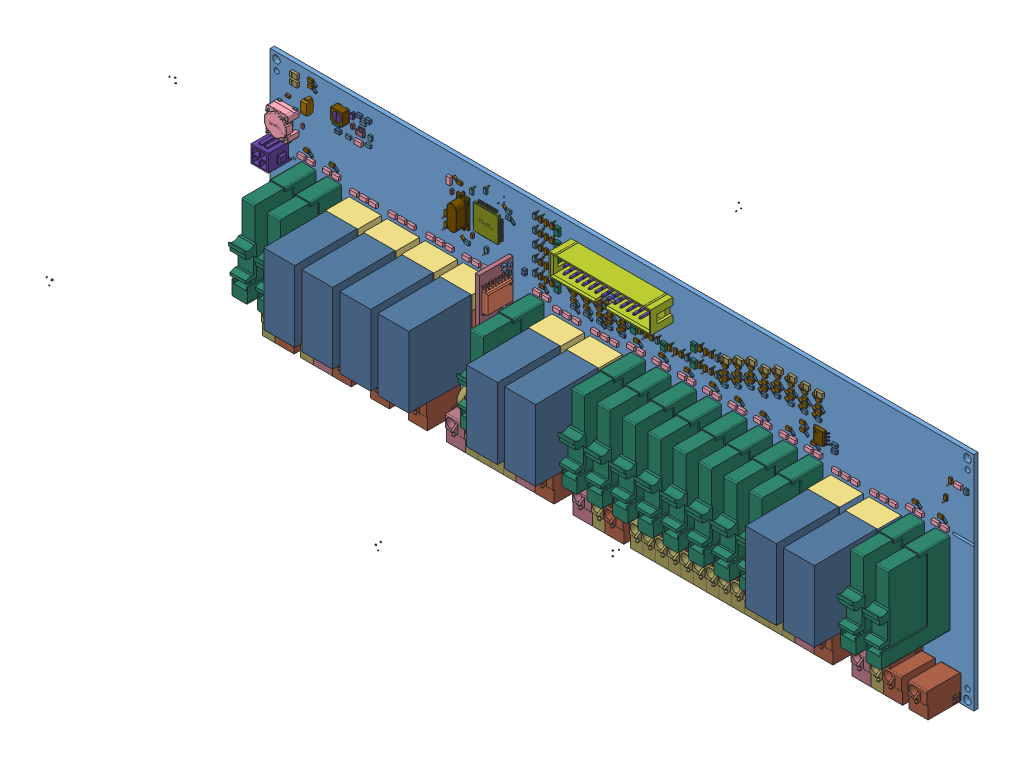
SolidWorks assembly _SC941C, configuration Default. Lengths in mm. (continued)
Components (placement in the parent): (continued)
- T27-1: T27 [Default] at origin size (320.25 73.48 23.48)
  - SW3dPS-transistor_SOT233_4-1: SW3dPS-transistor_SOT233_4 [Default] at (316.7762 70.6118 -21.9) x (1 0 0) z (0 -1 0) size (2.9 1.1 1.6)
  - SW3dPS-transistor_SOT233_5-1: SW3dPS-transistor_SOT233_5 [Default] at (0.3168 0.0706 -0.0219) x (1 0 0) z (0 -1 0) size (2.18 2.18 2.18)
  - SW3dPS-transistor_SOT233_6-1: SW3dPS-transistor_SOT233_6 [Default] at (0.0003 0.0001 0) x (1 0 0) z (0 -1 0) size (2.18 2.18 2.18)
  - SW3dPS-transistor_SOT233_7-1: SW3dPS-transistor_SOT233_7 [Default] x (1 0 0) z (0 -1 0) size (2.18 2.18 2.18)
- T24-1: T24 [Default] at origin size (297.39 73.44 23.48)
  - SW3dPS-transistor_SOT233_4-1: SW3dPS-transistor_SOT233_4 [Default] at (293.9162 70.5668 -21.9) x (1 0 0) z (0 -1 0) size (2.9 1.1 1.6)
  - SW3dPS-transistor_SOT233_5-1: SW3dPS-transistor_SOT233_5 [Default] at (0.2939 0.0706 -0.0219) x (1 0 0) z (0 -1 0) size (2.18 2.18 2.18)
  - SW3dPS-transistor_SOT233_6-1: SW3dPS-transistor_SOT233_6 [Default] at (0.0003 0.0001 0) x (1 0 0) z (0 -1 0) size (2.18 2.18 2.18)
  - SW3dPS-transistor_SOT233_7-1: SW3dPS-transistor_SOT233_7 [Default] x (1 0 0) z (0 -1 0) size (2.18 2.18 2.18)
- T25-1: T25 [Default] at origin size (305.01 73.44 23.48)
  - SW3dPS-transistor_SOT233_4-1: SW3dPS-transistor_SOT233_4 [Default] at (301.5362 70.5668 -21.9) x (1 0 0) z (0 -1 0) size (2.9 1.1 1.6)
  - SW3dPS-transistor_SOT233_5-1: SW3dPS-transistor_SOT233_5 [Default] at (0.3015 0.0706 -0.0219) x (1 0 0) z (0 -1 0) size (2.18 2.18 2.18)
  - SW3dPS-transistor_SOT233_6-1: SW3dPS-transistor_SOT233_6 [Default] at (0.0003 0.0001 0) x (1 0 0) z (0 -1 0) size (2.18 2.18 2.18)
  - SW3dPS-transistor_SOT233_7-1: SW3dPS-transistor_SOT233_7 [Default] x (1 0 0) z (0 -1 0) size (2.18 2.18 2.18)
- T14-1: T14 [Default] at origin size (200.87 73.48 23.48)
  - SW3dPS-transistor_SOT233_4-1: SW3dPS-transistor_SOT233_4 [Default] at (197.3962 70.6118 -21.9) x (1 0 0) z (0 -1 0) size (2.9 1.1 1.6)
  - SW3dPS-transistor_SOT233_5-1: SW3dPS-transistor_SOT233_5 [Default] at (0.1974 0.0706 -0.0219) x (1 0 0) z (0 -1 0) size (2.18 2.18 2.18)
  - SW3dPS-transistor_SOT233_6-1: SW3dPS-transistor_SOT233_6 [Default] at (0.0002 0.0001 0) x (1 0 0) z (0 -1 0) size (2.18 2.18 2.18)
  - SW3dPS-transistor_SOT233_7-1: SW3dPS-transistor_SOT233_7 [Default] x (1 0 0) z (0 -1 0) size (2.18 2.18 2.18)
- T15-1: T15 [Default] at origin size (208.49 73.48 23.48)
  - SW3dPS-transistor_SOT233_4-1: SW3dPS-transistor_SOT233_4 [Default] at (205.0162 70.6118 -21.9) x (1 0 0) z (0 -1 0) size (2.9 1.1 1.6)
  - SW3dPS-transistor_SOT233_5-1: SW3dPS-transistor_SOT233_5 [Default] at (0.205 0.0706 -0.0219) x (1 0 0) z (0 -1 0) size (2.18 2.18 2.18)
  - SW3dPS-transistor_SOT233_6-1: SW3dPS-transistor_SOT233_6 [Default] at (0.0002 0.0001 0) x (1 0 0) z (0 -1 0) size (2.18 2.18 2.18)
  - SW3dPS-transistor_SOT233_7-1: SW3dPS-transistor_SOT233_7 [Default] x (1 0 0) z (0 -1 0) size (2.18 2.18 2.18)
- T12-1: T12 [Default] at origin size (185.63 73.48 23.48)
  - SW3dPS-transistor_SOT233_4-1: SW3dPS-transistor_SOT233_4 [Default] at (182.1562 70.6118 -21.9) x (1 0 0) z (0 -1 0) size (2.9 1.1 1.6)
  - SW3dPS-transistor_SOT233_5-1: SW3dPS-transistor_SOT233_5 [Default] at (0.1822 0.0706 -0.0219) x (1 0 0) z (0 -1 0) size (2.18 2.18 2.18)
  - SW3dPS-transistor_SOT233_6-1: SW3dPS-transistor_SOT233_6 [Default] at (0.0002 0.0001 0) x (1 0 0) z (0 -1 0) size (2.18 2.18 2.18)
  - SW3dPS-transistor_SOT233_7-1: SW3dPS-transistor_SOT233_7 [Default] x (1 0 0) z (0 -1 0) size (2.18 2.18 2.18)
- T13-1: T13 [Default] at origin size (193.25 73.48 23.48)
  - SW3dPS-transistor_SOT233_4-1: SW3dPS-transistor_SOT233_4 [Default] at (189.7762 70.6118 -21.9) x (1 0 0) z (0 -1 0) size (2.9 1.1 1.6)
  - SW3dPS-transistor_SOT233_5-1: SW3dPS-transistor_SOT233_5 [Default] at (0.1898 0.0706 -0.0219) x (1 0 0) z (0 -1 0) size (2.18 2.18 2.18)
  - SW3dPS-transistor_SOT233_6-1: SW3dPS-transistor_SOT233_6 [Default] at (0.0002 0.0001 0) x (1 0 0) z (0 -1 0) size (2.18 2.18 2.18)
  - SW3dPS-transistor_SOT233_7-1: SW3dPS-transistor_SOT233_7 [Default] x (1 0 0) z (0 -1 0) size (2.18 2.18 2.18)
- T9-1: T9 [Default] at origin size (149.28 73.48 23.48)
  - SW3dPS-transistor_SOT233_4-1: SW3dPS-transistor_SOT233_4 [Default] at (145.8024 70.6118 -21.9) x (1 0 0) z (0 -1 0) size (2.9 1.1 1.6)
  - SW3dPS-transistor_SOT233_5-1: SW3dPS-transistor_SOT233_5 [Default] at (0.1458 0.0706 -0.0219) x (1 0 0) z (0 -1 0) size (2.18 2.18 2.18)
  - SW3dPS-transistor_SOT233_6-1: SW3dPS-transistor_SOT233_6 [Default] at (0.0001 0.0001 0) x (1 0 0) z (0 -1 0) size (2.18 2.18 2.18)
  - SW3dPS-transistor_SOT233_7-1: SW3dPS-transistor_SOT233_7 [Default] x (1 0 0) z (0 -1 0) size (2.18 2.18 2.18)
- T10-1: T10 [Default] at origin size (156.9 73.48 23.48)
  - SW3dPS-transistor_SOT233_4-1: SW3dPS-transistor_SOT233_4 [Default] at (153.4224 70.6118 -21.9) x (1 0 0) z (0 -1 0) size (2.9 1.1 1.6)
  - SW3dPS-transistor_SOT233_5-1: SW3dPS-transistor_SOT233_5 [Default] at (0.1534 0.0706 -0.0219) x (1 0 0) z (0 -1 0) size (2.18 2.18 2.18)
  - SW3dPS-transistor_SOT233_6-1: SW3dPS-transistor_SOT233_6 [Default] at (0.0002 0.0001 0) x (1 0 0) z (0 -1 0) size (2.18 2.18 2.18)
  - SW3dPS-transistor_SOT233_7-1: SW3dPS-transistor_SOT233_7 [Default] x (1 0 0) z (0 -1 0) size (2.18 2.18 2.18)
- T7_1-1: T7_1 [Default] at origin size (134.83 73.44 23.48)
  - SW3dPS-transistor_SOT233_4-1: SW3dPS-transistor_SOT233_4 [Default] at (131.3562 70.5668 -21.9) x (1 0 0) z (0 -1 0) size (2.9 1.1 1.6)
  - SW3dPS-transistor_SOT233_5-1: SW3dPS-transistor_SOT233_5 [Default] at (0.1314 0.0706 -0.0219) x (1 0 0) z (0 -1 0) size (2.18 2.18 2.18)
  - SW3dPS-transistor_SOT233_6-1: SW3dPS-transistor_SOT233_6 [Default] at (0.0001 0.0001 0) x (1 0 0) z (0 -1 0) size (2.18 2.18 2.18)
  - SW3dPS-transistor_SOT233_7-1: SW3dPS-transistor_SOT233_7 [Default] x (1 0 0) z (0 -1 0) size (2.18 2.18 2.18)
- T8-1: T8 [Default] at origin size (142.45 73.44 23.48)
  - SW3dPS-transistor_SOT233_4-1: SW3dPS-transistor_SOT233_4 [Default] at (138.9762 70.5668 -21.9) x (1 0 0) z (0 -1 0) size (2.9 1.1 1.6)
  - SW3dPS-transistor_SOT233_5-1: SW3dPS-transistor_SOT233_5 [Default] at (0.139 0.0706 -0.0219) x (1 0 0) z (0 -1 0) size (2.18 2.18 2.18)
  - SW3dPS-transistor_SOT233_6-1: SW3dPS-transistor_SOT233_6 [Default] at (0.0001 0.0001 0) x (1 0 0) z (0 -1 0) size (2.18 2.18 2.18)
  - SW3dPS-transistor_SOT233_7-1: SW3dPS-transistor_SOT233_7 [Default] x (1 0 0) z (0 -1 0) size (2.18 2.18 2.18)
- T5_1-1: T5_1 [Default] at origin size (119.59 73.44 23.48)
  - SW3dPS-transistor_SOT233_4-1: SW3dPS-transistor_SOT233_4 [Default] at (116.1162 70.5668 -21.9) x (1 0 0) z (0 -1 0) size (2.9 1.1 1.6)
  - SW3dPS-transistor_SOT233_5-1: SW3dPS-transistor_SOT233_5 [Default] at (0.1161 0.0706 -0.0219) x (1 0 0) z (0 -1 0) size (2.18 2.18 2.18)
  - SW3dPS-transistor_SOT233_6-1: SW3dPS-transistor_SOT233_6 [Default] at (0.0001 0.0001 0) x (1 0 0) z (0 -1 0) size (2.18 2.18 2.18)
  - SW3dPS-transistor_SOT233_7-1: SW3dPS-transistor_SOT233_7 [Default] x (1 0 0) z (0 -1 0) size (2.18 2.18 2.18)
- T6_1-1: T6_1 [Default] at origin size (127.21 73.44 23.48)
  - SW3dPS-transistor_SOT233_4-1: SW3dPS-transistor_SOT233_4 [Default] at (123.7362 70.5668 -21.9) x (1 0 0) z (0 -1 0) size (2.9 1.1 1.6)
  - SW3dPS-transistor_SOT233_5-1: SW3dPS-transistor_SOT233_5 [Default] at (0.1237 0.0706 -0.0219) x (1 0 0) z (0 -1 0) size (2.18 2.18 2.18)
  - SW3dPS-transistor_SOT233_6-1: SW3dPS-transistor_SOT233_6 [Default] at (0.0001 0.0001 0) x (1 0 0) z (0 -1 0) size (2.18 2.18 2.18)
  - SW3dPS-transistor_SOT233_7-1: SW3dPS-transistor_SOT233_7 [Default] x (1 0 0) z (0 -1 0) size (2.18 2.18 2.18)
- T3_1-1: T3_1 [Default] at origin size (104.35 73.44 23.48)
  - SW3dPS-transistor_SOT233_4-1: SW3dPS-transistor_SOT233_4 [Default] at (100.8762 70.5668 -21.9) x (1 0 0) z (0 -1 0) size (2.9 1.1 1.6)
  - SW3dPS-transistor_SOT233_5-1: SW3dPS-transistor_SOT233_5 [Default] at (0.1009 0.0706 -0.0219) x (1 0 0) z (0 -1 0) size (2.18 2.18 2.18)
  - SW3dPS-transistor_SOT233_6-1: SW3dPS-transistor_SOT233_6 [Default] at (0.0001 0.0001 0) x (1 0 0) z (0 -1 0) size (2.18 2.18 2.18)
  - SW3dPS-transistor_SOT233_7-1: SW3dPS-transistor_SOT233_7 [Default] x (1 0 0) z (0 -1 0) size (2.18 2.18 2.18)
- SUP_K19-1: SUP_K19 [Default] at origin size (13 30.3 9.5)
  - 1151724792-1: 1151724792 [Default] at (240.665 37.325 0) size (13 14.8 9.5)
    - Extruded_5-1: Extruded_5 [Default] at origin size (13 14.8 9.5)
  - 1151725064-1: 1151725064 [Default] at (240.665 24.925 5) size (13 10 4.5)
    - Extruded_6-1: Extruded_6 [Default] at origin size (13 10 4.5)
  - 1151724928-1: 1151724928 [Default] at (240.665 17.175 0) size (13 5.5 9.5)
    - Extruded_7-1: Extruded_7 [Default] at origin size (13 5.5 9.5)
- SUP_K18-1: SUP_K18 [Default] at origin size (13 30.3 9.5)
  - 1151724792-1: 1151724792 [Default] at (225.425 37.325 0) size (13 14.8 9.5)
    - Extruded_5-1: Extruded_5 [Default] at origin size (13 14.8 9.5)
  - 1151725064-1: 1151725064 [Default] at (225.425 24.925 5) size (13 10 4.5)
    - Extruded_6-1: Extruded_6 [Default] at origin size (13 10 4.5)
  - 1151724928-1: 1151724928 [Default] at (225.425 17.175 0) size (13 5.5 9.5)
    - Extruded_7-1: Extruded_7 [Default] at origin size (13 5.5 9.5)
- SUP_K6-1: SUP_K6 [Default] at origin size (13 30.3 9.5)
  - 1151724792-1: 1151724792 [Default] at (78.105 21.825 0) size (13 14.8 9.5)
    - Extruded_5-1: Extruded_5 [Default] at origin size (13 14.8 9.5)
  - 1151725064-1: 1151725064 [Default] at (78.105 34.225 5) size (13 10 4.5)
    - Extruded_6-1: Extruded_6 [Default] at origin size (13 10 4.5)
  - 1151724928-1: 1151724928 [Default] at (78.105 41.975 0) size (13 5.5 9.5)
    - Extruded_7-1: Extruded_7 [Default] at origin size (13 5.5 9.5)
- SUP_K5-1: SUP_K5 [Default] at origin size (13 30.3 9.5)
  - 1151724792-1: 1151724792 [Default] at (62.865 21.825 0) size (13 14.8 9.5)
    - Extruded_5-1: Extruded_5 [Default] at origin size (13 14.8 9.5)
  - 1151725064-1: 1151725064 [Default] at (62.865 34.225 5) size (13 10 4.5)
    - Extruded_6-1: Extruded_6 [Default] at origin size (13 10 4.5)
  - 1151724928-1: 1151724928 [Default] at (62.865 41.975 0) size (13 5.5 9.5)
    - Extruded_7-1: Extruded_7 [Default] at origin size (13 5.5 9.5)
- SUP_K4-1: SUP_K4 [Default] at origin size (13 30.3 9.5)
  - 1151724792-1: 1151724792 [Default] at (47.625 21.825 0) size (13 14.8 9.5)
    - Extruded_5-1: Extruded_5 [Default] at origin size (13 14.8 9.5)
  - 1151725064-1: 1151725064 [Default] at (47.625 34.225 5) size (13 10 4.5)
    - Extruded_6-1: Extruded_6 [Default] at origin size (13 10 4.5)
  - 1151724928-1: 1151724928 [Default] at (47.625 41.975 0) size (13 5.5 9.5)
    - Extruded_7-1: Extruded_7 [Default] at origin size (13 5.5 9.5)
- SUP_K3-1: SUP_K3 [Default] at origin size (13 30.3 9.5)
  - 1151724792-1: 1151724792 [Default] at (32.385 21.825 0) size (13 14.8 9.5)
    - Extruded_5-1: Extruded_5 [Default] at origin size (13 14.8 9.5)
  - 1151725064-1: 1151725064 [Default] at (32.385 34.225 5) size (13 10 4.5)
    - Extruded_6-1: Extruded_6 [Default] at origin size (13 10 4.5)
  - 1151724928-1: 1151724928 [Default] at (32.385 41.975 0) size (13 5.5 9.5)
    - Extruded_7-1: Extruded_7 [Default] at origin size (13 5.5 9.5)
- R86-1: R86 [Default] at origin size (3.3 1.97 0.78)
  - SW3dPS-0805_SMD_Resistor-1: SW3dPS-0805_SMD_Resistor [Default] at (192.7859 64.1349 0) x (-1 0 0) z (0 1 0) size (2 0.78 1.25)
  - 905261096-1: 905261096 [Default] at (194.5719 63.4603 0) size (1.03 1.35 0.76)
    - Extruded_2-1: Extruded_2 [Default] at origin size (1.03 1.35 0.76)
  - 905275240-1: 905275240 [Default] at (194.3338 63.5397 0) size (1.51 1.51 0.76)
    - Extruded_3-1: Extruded_3 [Default] at origin size (1.51 1.51 0.76)
  - 905265720-1: 905265720 [Default] at (194.4529 63.5 0) size (1.11 1.43 0.76)
    - Extruded_4-1: Extruded_4 [Default] at origin size (1.11 1.43 0.76)
- R82-1: R82 [Default] at origin size (3.3 1.97 0.78)
  - SW3dPS-0805_SMD_Resistor-1: SW3dPS-0805_SMD_Resistor [Default] at (197.9929 66.4209 0) x (-1 0 0) z (0 1 0) size (2 0.78 1.25)
  - 905261096-1: 905261096 [Default] at (199.7789 65.7463 0) size (1.03 1.35 0.76)
    - Extruded_2-1: Extruded_2 [Default] at origin size (1.03 1.35 0.76)
  - 905275240-1: 905275240 [Default] at (199.5408 65.8257 0) size (1.51 1.51 0.76)
    - Extruded_3-1: Extruded_3 [Default] at origin size (1.51 1.51 0.76)
  - 905265720-1: 905265720 [Default] at (199.6599 65.786 0) size (1.11 1.43 0.76)
    - Extruded_4-1: Extruded_4 [Default] at origin size (1.11 1.43 0.76)
- R90-1: R90 [Default] at origin size (1.97 3.3 0.78)
  - SW3dPS-0805_SMD_Resistor-1: SW3dPS-0805_SMD_Resistor [Default] at (265.4299 60.3251 0) x (0 1 0) z (1 0 0) size (2 0.78 1.25)
  - 905261640-1: 905261640 [Default] at (264.7553 58.5391 0) size (1.35 1.03 0.76)
    - Extruded_8-1: Extruded_8 [Default] at origin size (1.35 1.03 0.76)
  - 905260416-1: 905260416 [Default] at (264.8347 58.7772 0) size (1.51 1.51 0.76)
    - Extruded_9-1: Extruded_9 [Default] at origin size (1.51 1.51 0.76)
  - 905266128-1: 905266128 [Default] at (264.795 58.6581 0) size (1.43 1.11 0.76)
    - Extruded_10-1: Extruded_10 [Default] at origin size (1.43 1.11 0.76)
- R42-1: R42 [Default] at origin size (3.3 1.97 0.78)
  - SW3dPS-0805_SMD_Resistor-1: SW3dPS-0805_SMD_Resistor [Default] at (70.6121 72.1361 0) x (1 0 0) z (0 -1 0) size (2 0.78 1.25)
  - 905266264-1: 905266264 [Default] at (68.8261 72.8107 0) size (1.03 1.35 0.76)
    - Extruded_14-1: Extruded_14 [Default] at origin size (1.03 1.35 0.76)
  - 905263816-1: 905263816 [Default] at (69.0642 72.7313 0) size (1.51 1.51 0.76)
    - Extruded_15-1: Extruded_15 [Default] at origin size (1.51 1.51 0.76)
  - 905266536-1: 905266536 [Default] at (68.9451 72.771 0) size (1.11 1.43 0.76)
    - Extruded_16-1: Extruded_16 [Default] at origin size (1.11 1.43 0.76)
- R43-1: R43 [Default] at origin size (1.97 3.3 0.78)
  - SW3dPS-0805_SMD_Resistor-1: SW3dPS-0805_SMD_Resistor [Default] at (65.1509 54.8641 0) x (0 1 0) z (1 0 0) size (2 0.78 1.25)
  - 905261640-1: 905261640 [Default] at (64.4763 53.0781 0) size (1.35 1.03 0.76)
    - Extruded_8-1: Extruded_8 [Default] at origin size (1.35 1.03 0.76)
  - 905260416-1: 905260416 [Default] at (64.5557 53.3162 0) size (1.51 1.51 0.76)
    - Extruded_9-1: Extruded_9 [Default] at origin size (1.51 1.51 0.76)
  - 905266128-1: 905266128 [Default] at (64.516 53.1971 0) size (1.43 1.11 0.76)
    - Extruded_10-1: Extruded_10 [Default] at origin size (1.43 1.11 0.76)
- R44-1: R44 [Default] at origin size (1.97 3.3 0.78)
  - SW3dPS-0805_SMD_Resistor-1: SW3dPS-0805_SMD_Resistor [Default] at (65.1509 58.9281 0) x (0 1 0) z (1 0 0) size (2 0.78 1.25)
  - 905261640-1: 905261640 [Default] at (64.4763 57.1421 0) size (1.35 1.03 0.76)
    - Extruded_8-1: Extruded_8 [Default] at origin size (1.35 1.03 0.76)
  - 905260416-1: 905260416 [Default] at (64.5557 57.3802 0) size (1.51 1.51 0.76)
    - Extruded_9-1: Extruded_9 [Default] at origin size (1.51 1.51 0.76)
  - 905266128-1: 905266128 [Default] at (64.516 57.2611 0) size (1.43 1.11 0.76)
    - Extruded_10-1: Extruded_10 [Default] at origin size (1.43 1.11 0.76)
- R91-1: R91 [Default] at origin size (1.97 3.3 0.78)
  - SW3dPS-0805_SMD_Resistor-1: SW3dPS-0805_SMD_Resistor [Default] at (267.3349 67.1513 0) x (0 1 0) z (1 0 0) size (2 0.78 1.25)
  - 905261640-1: 905261640 [Default] at (266.6603 65.3653 0) size (1.35 1.03 0.76)
    - Extruded_8-1: Extruded_8 [Default] at origin size (1.35 1.03 0.76)
  - 905260416-1: 905260416 [Default] at (266.7397 65.6034 0) size (1.51 1.51 0.76)
    - Extruded_9-1: Extruded_9 [Default] at origin size (1.51 1.51 0.76)
  - 905266128-1: 905266128 [Default] at (266.7 65.4844 0) size (1.43 1.11 0.76)
    - Extruded_10-1: Extruded_10 [Default] at origin size (1.43 1.11 0.76)
- R87-1: R87 [Default] at origin size (3.3 1.97 0.78)
  - SW3dPS-0805_SMD_Resistor-1: SW3dPS-0805_SMD_Resistor [Default] at (192.7861 61.8491 0) x (1 0 0) z (0 -1 0) size (2 0.78 1.25)
  - 905266264-1: 905266264 [Default] at (191.0001 62.5237 0) size (1.03 1.35 0.76)
    - Extruded_14-1: Extruded_14 [Default] at origin size (1.03 1.35 0.76)
  - 905263816-1: 905263816 [Default] at (191.2382 62.4443 0) size (1.51 1.51 0.76)
    - Extruded_15-1: Extruded_15 [Default] at origin size (1.51 1.51 0.76)
  - 905266536-1: 905266536 [Default] at (191.1191 62.484 0) size (1.11 1.43 0.76)
    - Extruded_16-1: Extruded_16 [Default] at origin size (1.11 1.43 0.76)
- R83-1: R83 [Default] at origin size (3.3 1.97 0.78)
  - SW3dPS-0805_SMD_Resistor-1: SW3dPS-0805_SMD_Resistor [Default] at (197.9931 64.1351 0) x (1 0 0) z (0 -1 0) size (2 0.78 1.25)
  - 905266264-1: 905266264 [Default] at (196.2071 64.8097 0) size (1.03 1.35 0.76)
    - Extruded_14-1: Extruded_14 [Default] at origin size (1.03 1.35 0.76)
  - 905263816-1: 905263816 [Default] at (196.4452 64.7303 0) size (1.51 1.51 0.76)
    - Extruded_15-1: Extruded_15 [Default] at origin size (1.51 1.51 0.76)
  - 905266536-1: 905266536 [Default] at (196.3261 64.77 0) size (1.11 1.43 0.76)
    - Extruded_16-1: Extruded_16 [Default] at origin size (1.11 1.43 0.76)
- R88-1: R88 [Default] at origin size (3.3 1.97 0.78)
  - SW3dPS-0805_SMD_Resistor-1: SW3dPS-0805_SMD_Resistor [Default] at (192.7861 66.4211 0) x (1 0 0) z (0 -1 0) size (2 0.78 1.25)
  - 905266264-1: 905266264 [Default] at (191.0001 67.0957 0) size (1.03 1.35 0.76)
    - Extruded_14-1: Extruded_14 [Default] at origin size (1.03 1.35 0.76)
  - 905263816-1: 905263816 [Default] at (191.2382 67.0163 0) size (1.51 1.51 0.76)
    - Extruded_15-1: Extruded_15 [Default] at origin size (1.51 1.51 0.76)
  - 905266536-1: 905266536 [Default] at (191.1191 67.056 0) size (1.11 1.43 0.76)
    - Extruded_16-1: Extruded_16 [Default] at origin size (1.11 1.43 0.76)
- R84-1: R84 [Default] at origin size (3.3 1.97 0.78)
  - SW3dPS-0805_SMD_Resistor-1: SW3dPS-0805_SMD_Resistor [Default] at (197.9931 68.7071 0) x (1 0 0) z (0 -1 0) size (2 0.78 1.25)
  - 905266264-1: 905266264 [Default] at (196.2071 69.3817 0) size (1.03 1.35 0.76)
    - Extruded_14-1: Extruded_14 [Default] at origin size (1.03 1.35 0.76)
  - 905263816-1: 905263816 [Default] at (196.4452 69.3023 0) size (1.51 1.51 0.76)
    - Extruded_15-1: Extruded_15 [Default] at origin size (1.51 1.51 0.76)
  - 905266536-1: 905266536 [Default] at (196.3261 69.342 0) size (1.11 1.43 0.76)
    - Extruded_16-1: Extruded_16 [Default] at origin size (1.11 1.43 0.76)
- R3_1-1: R3_1 [Default] at origin size (3.3 1.97 0.78)
  - SW3dPS-0805_SMD_Resistor-1: SW3dPS-0805_SMD_Resistor [Default] at (10.8267 75.7079 0) x (-1 0 0) z (0 1 0) size (2 0.78 1.25)
  - 905261096-1: 905261096 [Default] at (12.6127 75.0333 0) size (1.03 1.35 0.76)
    - Extruded_2-1: Extruded_2 [Default] at origin size (1.03 1.35 0.76)
  - 905275240-1: 905275240 [Default] at (12.3746 75.1127 0) size (1.51 1.51 0.76)
    - Extruded_3-1: Extruded_3 [Default] at origin size (1.51 1.51 0.76)
  - 905265720-1: 905265720 [Default] at (12.4936 75.073 0) size (1.11 1.43 0.76)
    - Extruded_4-1: Extruded_4 [Default] at origin size (1.11 1.43 0.76)
- R1_1-1: R1_1 [Default] at origin size (3.3 1.97 0.78)
  - SW3dPS-0805_SMD_Resistor-1: SW3dPS-0805_SMD_Resistor [Default] at (10.8267 77.7716 0) x (-1 0 0) z (0 1 0) size (2 0.78 1.25)
  - 905261096-1: 905261096 [Default] at (12.6127 77.0971 0) size (1.03 1.35 0.76)
    - Extruded_2-1: Extruded_2 [Default] at origin size (1.03 1.35 0.76)
  - 905275240-1: 905275240 [Default] at (12.3746 77.1764 0) size (1.51 1.51 0.76)
    - Extruded_3-1: Extruded_3 [Default] at origin size (1.51 1.51 0.76)
  - 905265720-1: 905265720 [Default] at (12.4936 77.1367 0) size (1.11 1.43 0.76)
    - Extruded_4-1: Extruded_4 [Default] at origin size (1.11 1.43 0.76)
- R79-1: R79 [Default] at origin size (3.3 1.97 0.78)
  - SW3dPS-0805_SMD_Resistor-1: SW3dPS-0805_SMD_Resistor [Default] at (187.3249 64.1349 0) x (-1 0 0) z (0 1 0) size (2 0.78 1.25)
  - 905261096-1: 905261096 [Default] at (189.1109 63.4603 0) size (1.03 1.35 0.76)
    - Extruded_2-1: Extruded_2 [Default] at origin size (1.03 1.35 0.76)
  - 905275240-1: 905275240 [Default] at (188.8728 63.5397 0) size (1.51 1.51 0.76)
    - Extruded_3-1: Extruded_3 [Default] at origin size (1.51 1.51 0.76)
  - 905265720-1: 905265720 [Default] at (188.9919 63.5 0) size (1.11 1.43 0.76)
    - Extruded_4-1: Extruded_4 [Default] at origin size (1.11 1.43 0.76)
- R46-1: R46 [Default] at origin size (1.97 3.3 0.78)
  - SW3dPS-0805_SMD_Resistor-1: SW3dPS-0805_SMD_Resistor [Default] at (157.0989 56.8961 0) x (0 1 0) z (1 0 0) size (2 0.78 1.25)
  - 905261640-1: 905261640 [Default] at (156.4243 55.1101 0) size (1.35 1.03 0.76)
    - Extruded_8-1: Extruded_8 [Default] at origin size (1.35 1.03 0.76)
  - 905260416-1: 905260416 [Default] at (156.5037 55.3482 0) size (1.51 1.51 0.76)
    - Extruded_9-1: Extruded_9 [Default] at origin size (1.51 1.51 0.76)
  - 905266128-1: 905266128 [Default] at (156.464 55.2291 0) size (1.43 1.11 0.76)
    - Extruded_10-1: Extruded_10 [Default] at origin size (1.43 1.11 0.76)
- R29-1: R29 [Default] at origin size (3.3 1.97 0.78)
  - SW3dPS-0805_SMD_Resistor-1: SW3dPS-0805_SMD_Resistor [Default] at (126.6191 56.5151 0) x (1 0 0) z (0 -1 0) size (2 0.78 1.25)
  - 905266264-1: 905266264 [Default] at (124.8331 57.1897 0) size (1.03 1.35 0.76)
    - Extruded_14-1: Extruded_14 [Default] at origin size (1.03 1.35 0.76)
  - 905263816-1: 905263816 [Default] at (125.0712 57.1103 0) size (1.51 1.51 0.76)
    - Extruded_15-1: Extruded_15 [Default] at origin size (1.51 1.51 0.76)
  - 905266536-1: 905266536 [Default] at (124.9521 57.15 0) size (1.11 1.43 0.76)
    - Extruded_16-1: Extruded_16 [Default] at origin size (1.11 1.43 0.76)
- R31-1: R31 [Default] at origin size (1.97 3.3 0.78)
  - SW3dPS-0805_SMD_Resistor-1: SW3dPS-0805_SMD_Resistor [Default] at (105.2829 55.7531 0) x (0 1 0) z (1 0 0) size (2 0.78 1.25)
  - 905261640-1: 905261640 [Default] at (104.6083 53.9671 0) size (1.35 1.03 0.76)
    - Extruded_8-1: Extruded_8 [Default] at origin size (1.35 1.03 0.76)
  - 905260416-1: 905260416 [Default] at (104.6877 54.2052 0) size (1.51 1.51 0.76)
    - Extruded_9-1: Extruded_9 [Default] at origin size (1.51 1.51 0.76)
  - 905266128-1: 905266128 [Default] at (104.648 54.0861 0) size (1.43 1.11 0.76)
    - Extruded_10-1: Extruded_10 [Default] at origin size (1.43 1.11 0.76)
- R24-1: R24 [Default] at origin size (1.97 3.3 0.78)
  - SW3dPS-0805_SMD_Resistor-1: SW3dPS-0805_SMD_Resistor [Default] at (105.2829 75.5651 0) x (0 1 0) z (1 0 0) size (2 0.78 1.25)
  - 905261640-1: 905261640 [Default] at (104.6083 73.7791 0) size (1.35 1.03 0.76)
    - Extruded_8-1: Extruded_8 [Default] at origin size (1.35 1.03 0.76)
  - 905260416-1: 905260416 [Default] at (104.6877 74.0172 0) size (1.51 1.51 0.76)
    - Extruded_9-1: Extruded_9 [Default] at origin size (1.51 1.51 0.76)
  - 905266128-1: 905266128 [Default] at (104.648 73.8981 0) size (1.43 1.11 0.76)
    - Extruded_10-1: Extruded_10 [Default] at origin size (1.43 1.11 0.76)
- R19_1-1: R19_1 [Default] at origin size (1.97 3.3 0.78)
  - SW3dPS-0805_SMD_Resistor-1: SW3dPS-0805_SMD_Resistor [Default] at (105.2829 65.6591 0) x (0 1 0) z (1 0 0) size (2 0.78 1.25)
  - 905261640-1: 905261640 [Default] at (104.6083 63.8731 0) size (1.35 1.03 0.76)
    - Extruded_8-1: Extruded_8 [Default] at origin size (1.35 1.03 0.76)
  - 905260416-1: 905260416 [Default] at (104.6877 64.1112 0) size (1.51 1.51 0.76)
    - Extruded_9-1: Extruded_9 [Default] at origin size (1.51 1.51 0.76)
  - 905266128-1: 905266128 [Default] at (104.648 63.9921 0) size (1.43 1.11 0.76)
    - Extruded_10-1: Extruded_10 [Default] at origin size (1.43 1.11 0.76)
- R13-1: R13 [Default] at origin size (1.97 3.3 0.78)
  - SW3dPS-0805_SMD_Resistor-1: SW3dPS-0805_SMD_Resistor [Default] at (105.2829 70.6121 0) x (0 1 0) z (1 0 0) size (2 0.78 1.25)
  - 905261640-1: 905261640 [Default] at (104.6083 68.8261 0) size (1.35 1.03 0.76)
    - Extruded_8-1: Extruded_8 [Default] at origin size (1.35 1.03 0.76)
  - 905260416-1: 905260416 [Default] at (104.6877 69.0642 0) size (1.51 1.51 0.76)
    - Extruded_9-1: Extruded_9 [Default] at origin size (1.51 1.51 0.76)
  - 905266128-1: 905266128 [Default] at (104.648 68.9451 0) size (1.43 1.11 0.76)
    - Extruded_10-1: Extruded_10 [Default] at origin size (1.43 1.11 0.76)
- R76-1: R76 [Default] at origin size (3.3 1.97 0.78)
  - SW3dPS-0805_SMD_Resistor-1: SW3dPS-0805_SMD_Resistor [Default] at (203.4539 66.4209 0) x (-1 0 0) z (0 1 0) size (2 0.78 1.25)
  - 905261096-1: 905261096 [Default] at (205.2399 65.7463 0) size (1.03 1.35 0.76)
    - Extruded_2-1: Extruded_2 [Default] at origin size (1.03 1.35 0.76)
  - 905275240-1: 905275240 [Default] at (205.0018 65.8257 0) size (1.51 1.51 0.76)
    - Extruded_3-1: Extruded_3 [Default] at origin size (1.51 1.51 0.76)
  - 905265720-1: 905265720 [Default] at (205.1209 65.786 0) size (1.11 1.43 0.76)
    - Extruded_4-1: Extruded_4 [Default] at origin size (1.11 1.43 0.76)
- R73-1: R73 [Default] at origin size (3.3 1.97 0.78)
  - SW3dPS-0805_SMD_Resistor-1: SW3dPS-0805_SMD_Resistor [Default] at (182.1179 61.8489 0) x (-1 0 0) z (0 1 0) size (2 0.78 1.25)
  - 905261096-1: 905261096 [Default] at (183.9039 61.1743 0) size (1.03 1.35 0.76)
    - Extruded_2-1: Extruded_2 [Default] at origin size (1.03 1.35 0.76)
  - 905275240-1: 905275240 [Default] at (183.6658 61.2537 0) size (1.51 1.51 0.76)
    - Extruded_3-1: Extruded_3 [Default] at origin size (1.51 1.51 0.76)
  - 905265720-1: 905265720 [Default] at (183.7849 61.214 0) size (1.11 1.43 0.76)
    - Extruded_4-1: Extruded_4 [Default] at origin size (1.11 1.43 0.76)
- R67-1: R67 [Default] at origin size (3.3 1.97 0.78)
  - SW3dPS-0805_SMD_Resistor-1: SW3dPS-0805_SMD_Resistor [Default] at (208.9149 66.4209 0) x (-1 0 0) z (0 1 0) size (2 0.78 1.25)
  - 905261096-1: 905261096 [Default] at (210.7009 65.7463 0) size (1.03 1.35 0.76)
    - Extruded_2-1: Extruded_2 [Default] at origin size (1.03 1.35 0.76)
  - 905275240-1: 905275240 [Default] at (210.4628 65.8257 0) size (1.51 1.51 0.76)
    - Extruded_3-1: Extruded_3 [Default] at origin size (1.51 1.51 0.76)
  - 905265720-1: 905265720 [Default] at (210.5819 65.786 0) size (1.11 1.43 0.76)
    - Extruded_4-1: Extruded_4 [Default] at origin size (1.11 1.43 0.76)
- R80-1: R80 [Default] at origin size (3.3 1.97 0.78)
  - SW3dPS-0805_SMD_Resistor-1: SW3dPS-0805_SMD_Resistor [Default] at (187.3251 61.8491 0) x (1 0 0) z (0 -1 0) size (2 0.78 1.25)
  - 905266264-1: 905266264 [Default] at (185.5391 62.5237 0) size (1.03 1.35 0.76)
    - Extruded_14-1: Extruded_14 [Default] at origin size (1.03 1.35 0.76)
  - 905263816-1: 905263816 [Default] at (185.7772 62.4443 0) size (1.51 1.51 0.76)
    - Extruded_15-1: Extruded_15 [Default] at origin size (1.51 1.51 0.76)
  - 905266536-1: 905266536 [Default] at (185.6581 62.484 0) size (1.11 1.43 0.76)
    - Extruded_16-1: Extruded_16 [Default] at origin size (1.11 1.43 0.76)
- R77-1: R77 [Default] at origin size (3.3 1.97 0.78)
  - SW3dPS-0805_SMD_Resistor-1: SW3dPS-0805_SMD_Resistor [Default] at (203.4541 64.1351 0) x (1 0 0) z (0 -1 0) size (2 0.78 1.25)
  - 905266264-1: 905266264 [Default] at (201.6681 64.8097 0) size (1.03 1.35 0.76)
    - Extruded_14-1: Extruded_14 [Default] at origin size (1.03 1.35 0.76)
  - 905263816-1: 905263816 [Default] at (201.9062 64.7303 0) size (1.51 1.51 0.76)
    - Extruded_15-1: Extruded_15 [Default] at origin size (1.51 1.51 0.76)
  - 905266536-1: 905266536 [Default] at (201.7871 64.77 0) size (1.11 1.43 0.76)
    - Extruded_16-1: Extruded_16 [Default] at origin size (1.11 1.43 0.76)
- R74-1: R74 [Default] at origin size (3.3 1.97 0.78)
  - SW3dPS-0805_SMD_Resistor-1: SW3dPS-0805_SMD_Resistor [Default] at (182.1181 59.5631 0) x (1 0 0) z (0 -1 0) size (2 0.78 1.25)
  - 905266264-1: 905266264 [Default] at (180.3321 60.2377 0) size (1.03 1.35 0.76)
    - Extruded_14-1: Extruded_14 [Default] at origin size (1.03 1.35 0.76)
  - 905263816-1: 905263816 [Default] at (180.5702 60.1583 0) size (1.51 1.51 0.76)
    - Extruded_15-1: Extruded_15 [Default] at origin size (1.51 1.51 0.76)
  - 905266536-1: 905266536 [Default] at (180.4511 60.198 0) size (1.11 1.43 0.76)
    - Extruded_16-1: Extruded_16 [Default] at origin size (1.11 1.43 0.76)
- R68-1: R68 [Default] at origin size (3.3 1.97 0.78)
  - SW3dPS-0805_SMD_Resistor-1: SW3dPS-0805_SMD_Resistor [Default] at (208.9151 64.1351 0) x (1 0 0) z (0 -1 0) size (2 0.78 1.25)
  - 905266264-1: 905266264 [Default] at (207.1291 64.8097 0) size (1.03 1.35 0.76)
    - Extruded_14-1: Extruded_14 [Default] at origin size (1.03 1.35 0.76)
  - 905263816-1: 905263816 [Default] at (207.3672 64.7303 0) size (1.51 1.51 0.76)
    - Extruded_15-1: Extruded_15 [Default] at origin size (1.51 1.51 0.76)
  - 905266536-1: 905266536 [Default] at (207.2481 64.77 0) size (1.11 1.43 0.76)
    - Extruded_16-1: Extruded_16 [Default] at origin size (1.11 1.43 0.76)
- R81-1: R81 [Default] at origin size (3.3 1.97 0.78)
  - SW3dPS-0805_SMD_Resistor-1: SW3dPS-0805_SMD_Resistor [Default] at (187.3251 66.4211 0) x (1 0 0) z (0 -1 0) size (2 0.78 1.25)
  - 905266264-1: 905266264 [Default] at (185.5391 67.0957 0) size (1.03 1.35 0.76)
    - Extruded_14-1: Extruded_14 [Default] at origin size (1.03 1.35 0.76)
  - 905263816-1: 905263816 [Default] at (185.7772 67.0163 0) size (1.51 1.51 0.76)
    - Extruded_15-1: Extruded_15 [Default] at origin size (1.51 1.51 0.76)
  - 905266536-1: 905266536 [Default] at (185.6581 67.056 0) size (1.11 1.43 0.76)
    - Extruded_16-1: Extruded_16 [Default] at origin size (1.11 1.43 0.76)
- R78-1: R78 [Default] at origin size (3.3 1.97 0.78)
  - SW3dPS-0805_SMD_Resistor-1: SW3dPS-0805_SMD_Resistor [Default] at (203.4541 68.7071 0) x (1 0 0) z (0 -1 0) size (2 0.78 1.25)
  - 905266264-1: 905266264 [Default] at (201.6681 69.3817 0) size (1.03 1.35 0.76)
    - Extruded_14-1: Extruded_14 [Default] at origin size (1.03 1.35 0.76)
  - 905263816-1: 905263816 [Default] at (201.9062 69.3023 0) size (1.51 1.51 0.76)
    - Extruded_15-1: Extruded_15 [Default] at origin size (1.51 1.51 0.76)
  - 905266536-1: 905266536 [Default] at (201.7871 69.342 0) size (1.11 1.43 0.76)
    - Extruded_16-1: Extruded_16 [Default] at origin size (1.11 1.43 0.76)
- R75-1: R75 [Default] at origin size (3.3 1.97 0.78)
  - SW3dPS-0805_SMD_Resistor-1: SW3dPS-0805_SMD_Resistor [Default] at (182.1181 64.1351 0) x (1 0 0) z (0 -1 0) size (2 0.78 1.25)
  - 905266264-1: 905266264 [Default] at (180.3321 64.8097 0) size (1.03 1.35 0.76)
    - Extruded_14-1: Extruded_14 [Default] at origin size (1.03 1.35 0.76)
  - 905263816-1: 905263816 [Default] at (180.5702 64.7303 0) size (1.51 1.51 0.76)
    - Extruded_15-1: Extruded_15 [Default] at origin size (1.51 1.51 0.76)
  - 905266536-1: 905266536 [Default] at (180.4511 64.77 0) size (1.11 1.43 0.76)
    - Extruded_16-1: Extruded_16 [Default] at origin size (1.11 1.43 0.76)
- R69-1: R69 [Default] at origin size (3.3 1.97 0.78)
  - SW3dPS-0805_SMD_Resistor-1: SW3dPS-0805_SMD_Resistor [Default] at (208.9151 68.7071 0) x (1 0 0) z (0 -1 0) size (2 0.78 1.25)
  - 905266264-1: 905266264 [Default] at (207.1291 69.3817 0) size (1.03 1.35 0.76)
    - Extruded_14-1: Extruded_14 [Default] at origin size (1.03 1.35 0.76)
  - 905263816-1: 905263816 [Default] at (207.3672 69.3023 0) size (1.51 1.51 0.76)
    - Extruded_15-1: Extruded_15 [Default] at origin size (1.51 1.51 0.76)
  - 905266536-1: 905266536 [Default] at (207.2481 69.342 0) size (1.11 1.43 0.76)
    - Extruded_16-1: Extruded_16 [Default] at origin size (1.11 1.43 0.76)
- R62-1: R62 [Default] at origin size (3.3 1.97 0.78)
  - SW3dPS-0805_SMD_Resistor-1: SW3dPS-0805_SMD_Resistor [Default] at (176.9109 59.5629 0) x (-1 0 0) z (0 1 0) size (2 0.78 1.25)
  - 905261096-1: 905261096 [Default] at (178.6969 58.8883 0) size (1.03 1.35 0.76)
    - Extruded_2-1: Extruded_2 [Default] at origin size (1.03 1.35 0.76)
  - 905275240-1: 905275240 [Default] at (178.4588 58.9677 0) size (1.51 1.51 0.76)
    - Extruded_3-1: Extruded_3 [Default] at origin size (1.51 1.51 0.76)
  - 905265720-1: 905265720 [Default] at (178.5779 58.928 0) size (1.11 1.43 0.76)
    - Extruded_4-1: Extruded_4 [Default] at origin size (1.11 1.43 0.76)
- R58-1: R58 [Default] at origin size (3.3 1.97 0.78)
  - SW3dPS-0805_SMD_Resistor-1: SW3dPS-0805_SMD_Resistor [Default] at (214.3759 66.4209 0) x (-1 0 0) z (0 1 0) size (2 0.78 1.25)
  - 905261096-1: 905261096 [Default] at (216.1619 65.7463 0) size (1.03 1.35 0.76)
    - Extruded_2-1: Extruded_2 [Default] at origin size (1.03 1.35 0.76)
  - 905275240-1: 905275240 [Default] at (215.9238 65.8257 0) size (1.51 1.51 0.76)
    - Extruded_3-1: Extruded_3 [Default] at origin size (1.51 1.51 0.76)
  - 905265720-1: 905265720 [Default] at (216.0429 65.786 0) size (1.11 1.43 0.76)
    - Extruded_4-1: Extruded_4 [Default] at origin size (1.11 1.43 0.76)
- R54-1: R54 [Default] at origin size (1.97 3.3 0.78)
  - SW3dPS-0805_SMD_Resistor-1: SW3dPS-0805_SMD_Resistor [Default] at (169.1639 62.7381 0) x (0 1 0) z (1 0 0) size (2 0.78 1.25)
  - 905261640-1: 905261640 [Default] at (168.4893 60.9521 0) size (1.35 1.03 0.76)
    - Extruded_8-1: Extruded_8 [Default] at origin size (1.35 1.03 0.76)
  - 905260416-1: 905260416 [Default] at (168.5687 61.1902 0) size (1.51 1.51 0.76)
    - Extruded_9-1: Extruded_9 [Default] at origin size (1.51 1.51 0.76)
  - 905266128-1: 905266128 [Default] at (168.529 61.0711 0) size (1.43 1.11 0.76)
    - Extruded_10-1: Extruded_10 [Default] at origin size (1.43 1.11 0.76)
- R50-1: R50 [Default] at origin size (1.97 3.3 0.78)
  - SW3dPS-0805_SMD_Resistor-1: SW3dPS-0805_SMD_Resistor [Default] at (169.0369 56.8961 0) x (0 1 0) z (1 0 0) size (2 0.78 1.25)
  - 905261640-1: 905261640 [Default] at (168.3623 55.1101 0) size (1.35 1.03 0.76)
    - Extruded_8-1: Extruded_8 [Default] at origin size (1.35 1.03 0.76)
  - 905260416-1: 905260416 [Default] at (168.4417 55.3482 0) size (1.51 1.51 0.76)
    - Extruded_9-1: Extruded_9 [Default] at origin size (1.51 1.51 0.76)
  - 905266128-1: 905266128 [Default] at (168.402 55.2291 0) size (1.43 1.11 0.76)
    - Extruded_10-1: Extruded_10 [Default] at origin size (1.43 1.11 0.76)
- R64-1: R64 [Default] at origin size (3.3 1.97 0.78)
  - SW3dPS-0805_SMD_Resistor-1: SW3dPS-0805_SMD_Resistor [Default] at (176.9111 57.2771 0) x (1 0 0) z (0 -1 0) size (2 0.78 1.25)
  - 905266264-1: 905266264 [Default] at (175.1251 57.9517 0) size (1.03 1.35 0.76)
    - Extruded_14-1: Extruded_14 [Default] at origin size (1.03 1.35 0.76)
  - 905263816-1: 905263816 [Default] at (175.3632 57.8723 0) size (1.51 1.51 0.76)
    - Extruded_15-1: Extruded_15 [Default] at origin size (1.51 1.51 0.76)
  - 905266536-1: 905266536 [Default] at (175.2441 57.912 0) size (1.11 1.43 0.76)
    - Extruded_16-1: Extruded_16 [Default] at origin size (1.11 1.43 0.76)
- R59-1: R59 [Default] at origin size (3.3 1.97 0.78)
  - SW3dPS-0805_SMD_Resistor-1: SW3dPS-0805_SMD_Resistor [Default] at (214.3761 64.1351 0) x (1 0 0) z (0 -1 0) size (2 0.78 1.25)
  - 905266264-1: 905266264 [Default] at (212.5901 64.8097 0) size (1.03 1.35 0.76)
    - Extruded_14-1: Extruded_14 [Default] at origin size (1.03 1.35 0.76)
  - 905263816-1: 905263816 [Default] at (212.8282 64.7303 0) size (1.51 1.51 0.76)
    - Extruded_15-1: Extruded_15 [Default] at origin size (1.51 1.51 0.76)
  - 905266536-1: 905266536 [Default] at (212.7091 64.77 0) size (1.11 1.43 0.76)
    - Extruded_16-1: Extruded_16 [Default] at origin size (1.11 1.43 0.76)
- R55-1: R55 [Default] at origin size (1.97 3.3 0.78)
  - SW3dPS-0805_SMD_Resistor-1: SW3dPS-0805_SMD_Resistor [Default] at (171.4501 62.7379 0) x (0 -1 0) z (-1 0 0) size (2 0.78 1.25)
  - 905262864-1: 905262864 [Default] at (172.1247 64.5239 0) size (1.35 1.03 0.76)
    - Extruded_11-1: Extruded_11 [Default] at origin size (1.35 1.03 0.76)
  - 905261368-1: 905261368 [Default] at (172.0453 64.2858 0) size (1.51 1.51 0.76)
    - Extruded_12-1: Extruded_12 [Default] at origin size (1.51 1.51 0.76)
  - 905260688-1: 905260688 [Default] at (172.085 64.4049 0) size (1.43 1.11 0.76)
    - Extruded_13-1: Extruded_13 [Default] at origin size (1.43 1.11 0.76)
- R51-1: R51 [Default] at origin size (1.97 3.3 0.78)
  - SW3dPS-0805_SMD_Resistor-1: SW3dPS-0805_SMD_Resistor [Default] at (171.3231 56.8959 0) x (0 -1 0) z (-1 0 0) size (2 0.78 1.25)
  - 905262864-1: 905262864 [Default] at (171.9977 58.6819 0) size (1.35 1.03 0.76)
    - Extruded_11-1: Extruded_11 [Default] at origin size (1.35 1.03 0.76)
  - 905261368-1: 905261368 [Default] at (171.9183 58.4438 0) size (1.51 1.51 0.76)
    - Extruded_12-1: Extruded_12 [Default] at origin size (1.51 1.51 0.76)
  - 905260688-1: 905260688 [Default] at (171.958 58.5629 0) size (1.43 1.11 0.76)
    - Extruded_13-1: Extruded_13 [Default] at origin size (1.43 1.11 0.76)
- R65-1: R65 [Default] at origin size (3.3 1.97 0.78)
  - SW3dPS-0805_SMD_Resistor-1: SW3dPS-0805_SMD_Resistor [Default] at (176.9111 61.8491 0) x (1 0 0) z (0 -1 0) size (2 0.78 1.25)
  - 905266264-1: 905266264 [Default] at (175.1251 62.5237 0) size (1.03 1.35 0.76)
    - Extruded_14-1: Extruded_14 [Default] at origin size (1.03 1.35 0.76)
  - 905263816-1: 905263816 [Default] at (175.3632 62.4443 0) size (1.51 1.51 0.76)
    - Extruded_15-1: Extruded_15 [Default] at origin size (1.51 1.51 0.76)
  - 905266536-1: 905266536 [Default] at (175.2441 62.484 0) size (1.11 1.43 0.76)
    - Extruded_16-1: Extruded_16 [Default] at origin size (1.11 1.43 0.76)
- R61-1: R61 [Default] at origin size (3.3 1.97 0.78)
  - SW3dPS-0805_SMD_Resistor-1: SW3dPS-0805_SMD_Resistor [Default] at (214.3761 68.7071 0) x (1 0 0) z (0 -1 0) size (2 0.78 1.25)
  - 905266264-1: 905266264 [Default] at (212.5901 69.3817 0) size (1.03 1.35 0.76)
    - Extruded_14-1: Extruded_14 [Default] at origin size (1.03 1.35 0.76)
  - 905263816-1: 905263816 [Default] at (212.8282 69.3023 0) size (1.51 1.51 0.76)
    - Extruded_15-1: Extruded_15 [Default] at origin size (1.51 1.51 0.76)
  - 905266536-1: 905266536 [Default] at (212.7091 69.342 0) size (1.11 1.43 0.76)
    - Extruded_16-1: Extruded_16 [Default] at origin size (1.11 1.43 0.76)
- R57-1: R57 [Default] at origin size (1.97 3.3 0.78)
  - SW3dPS-0805_SMD_Resistor-1: SW3dPS-0805_SMD_Resistor [Default] at (166.8781 62.7379 0) x (0 -1 0) z (-1 0 0) size (2 0.78 1.25)
  - 905262864-1: 905262864 [Default] at (167.5527 64.5239 0) size (1.35 1.03 0.76)
    - Extruded_11-1: Extruded_11 [Default] at origin size (1.35 1.03 0.76)
  - 905261368-1: 905261368 [Default] at (167.4733 64.2858 0) size (1.51 1.51 0.76)
    - Extruded_12-1: Extruded_12 [Default] at origin size (1.51 1.51 0.76)
  - 905260688-1: 905260688 [Default] at (167.513 64.4049 0) size (1.43 1.11 0.76)
    - Extruded_13-1: Extruded_13 [Default] at origin size (1.43 1.11 0.76)
- R53-1: R53 [Default] at origin size (1.97 3.3 0.78)
  - SW3dPS-0805_SMD_Resistor-1: SW3dPS-0805_SMD_Resistor [Default] at (166.7511 56.8959 0) x (0 -1 0) z (-1 0 0) size (2 0.78 1.25)
  - 905262864-1: 905262864 [Default] at (167.4257 58.6819 0) size (1.35 1.03 0.76)
    - Extruded_11-1: Extruded_11 [Default] at origin size (1.35 1.03 0.76)
  - 905261368-1: 905261368 [Default] at (167.3463 58.4438 0) size (1.51 1.51 0.76)
    - Extruded_12-1: Extruded_12 [Default] at origin size (1.51 1.51 0.76)
  - 905260688-1: 905260688 [Default] at (167.386 58.5629 0) size (1.43 1.11 0.76)
    - Extruded_13-1: Extruded_13 [Default] at origin size (1.43 1.11 0.76)
- R41-1: R41 [Default] at origin size (1.97 3.3 0.78)
  - SW3dPS-0805_SMD_Resistor-1: SW3dPS-0805_SMD_Resistor [Default] at (145.1609 56.8961 0) x (0 1 0) z (1 0 0) size (2 0.78 1.25)
  - 905261640-1: 905261640 [Default] at (144.4863 55.1101 0) size (1.35 1.03 0.76)
    - Extruded_8-1: Extruded_8 [Default] at origin size (1.35 1.03 0.76)
  - 905260416-1: 905260416 [Default] at (144.5657 55.3482 0) size (1.51 1.51 0.76)
    - Extruded_9-1: Extruded_9 [Default] at origin size (1.51 1.51 0.76)
  - 905266128-1: 905266128 [Default] at (144.526 55.2291 0) size (1.43 1.11 0.76)
    - Extruded_10-1: Extruded_10 [Default] at origin size (1.43 1.11 0.76)
- R37-1: R37 [Default] at origin size (3.3 1.97 0.78)
  - SW3dPS-0805_SMD_Resistor-1: SW3dPS-0805_SMD_Resistor [Default] at (130.8099 56.5149 0) x (-1 0 0) z (0 1 0) size (2 0.78 1.25)
  - 905261096-1: 905261096 [Default] at (132.5959 55.8403 0) size (1.03 1.35 0.76)
    - Extruded_2-1: Extruded_2 [Default] at origin size (1.03 1.35 0.76)
  - 905275240-1: 905275240 [Default] at (132.3578 55.9197 0) size (1.51 1.51 0.76)
    - Extruded_3-1: Extruded_3 [Default] at origin size (1.51 1.51 0.76)
  - 905265720-1: 905265720 [Default] at (132.4769 55.88 0) size (1.11 1.43 0.76)
    - Extruded_4-1: Extruded_4 [Default] at origin size (1.11 1.43 0.76)
- R34-1: R34 [Default] at origin size (3.3 1.97 0.78)
  - SW3dPS-0805_SMD_Resistor-1: SW3dPS-0805_SMD_Resistor [Default] at (136.0169 56.5149 0) x (-1 0 0) z (0 1 0) size (2 0.78 1.25)
  - 905261096-1: 905261096 [Default] at (137.8029 55.8403 0) size (1.03 1.35 0.76)
    - Extruded_2-1: Extruded_2 [Default] at origin size (1.03 1.35 0.76)
  - 905275240-1: 905275240 [Default] at (137.5648 55.9197 0) size (1.51 1.51 0.76)
    - Extruded_3-1: Extruded_3 [Default] at origin size (1.51 1.51 0.76)
  - 905265720-1: 905265720 [Default] at (137.6839 55.88 0) size (1.11 1.43 0.76)
    - Extruded_4-1: Extruded_4 [Default] at origin size (1.11 1.43 0.76)
